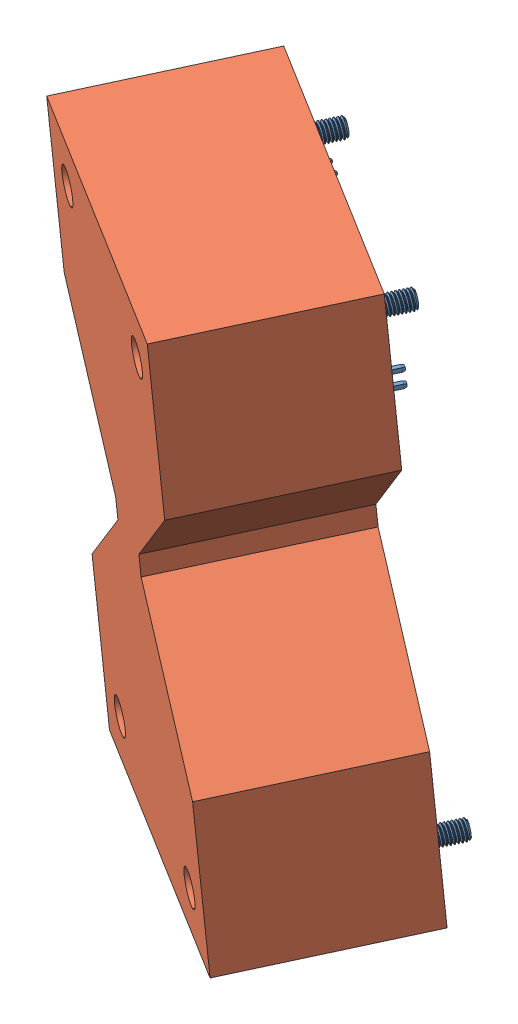
SolidWorks assembly 装配体1, configuration 默认. Lengths in mm.
Overall size (62.52 101.43 63.71).
2 component instances, 2 part files, 3 mates.
Components (placement in the parent):
- 电路板-1: 电路板 [默认] at (133.9666 -10.9268 -34.1234) x (0.853532 -0.024247 0.520477) z (0.520477 0.086162 -0.849518) size (46 92 16.42)
- 外壳-下-1: 外壳-下 [默认] at (120.018 -13.236 -11.3562) x (0.853532 -0.024247 0.520477) z (-0.024247 0.995986 0.086162) size (52 29.8 98)
Mates (geometry in assembly coordinates):
- 平行2: parallel aligned: plane of 电路板-1 through (154.7132 -57.2998 -26.1159) normal (0.520477 0.086162 -0.849518); plane of 外壳-下-1 through (120.018 -13.236 -11.3562) normal (0.520477 0.086162 -0.849518)
- 重合5: coincident aligned: line of 电路板-1 through (152.0799 -54.2391 -27.4188) axis (0.024247 -0.995986 -0.086162); line of 外壳-下-1 through (152.0799 -54.239 -27.4188) axis (0.024247 -0.995986 -0.086162)
- 重合6: coincident anti-aligned: plane of 电路板-1 through (172.9045 -12.0959 -9.6516) normal (-0.024247 0.995986 0.086162); plane of 外壳-下-1 through (133.9668 -10.9268 -34.1233) normal (0.024247 -0.995986 -0.086162)
